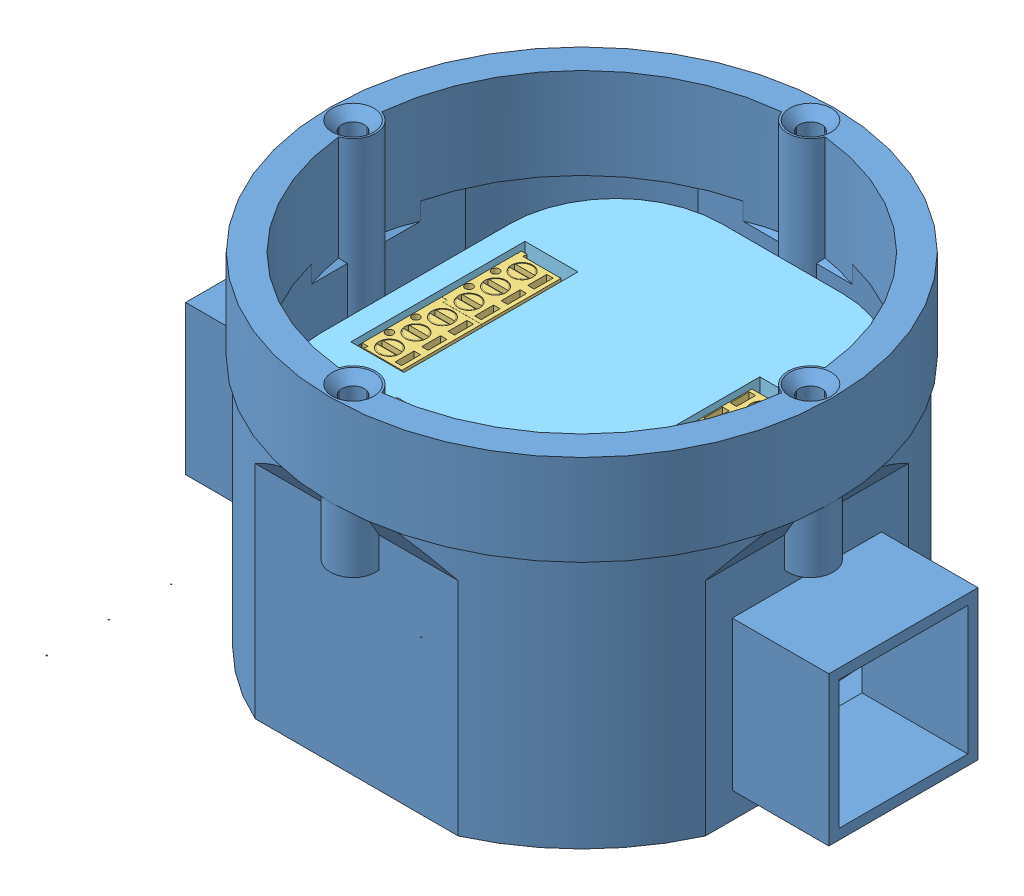
SolidWorks assembly Сборка смартбокса в подрозетнике, configuration Default. Lengths in mm.
Overall size (84.94 45.2 92.53).
6 component instances, 5 part files, 4 mates.
Components (placement in the parent):
- Подрозетник, реинкарнация-1: Подрозетник, реинкарнация [Default] at (-100.2738 -11.9044 46.462) size (84.94 45.2 66.4)
- Сборка плат смарт-бокса-1: Сборка плат смарт-бокса [Default] at (-98.3986 -21.5594 77.5072) x (0 0 1) z (0 1 0) size (85.93 44 32.41)
  - Плата смарт-бокса 1-1: Плата смарт-бокса 1 [Default] at (-165.9192 -27.3465 18.5165) size (50.47 38.8 18.8)
  - Плата смарт-бокса 2-1: Плата смарт-бокса 2 [Default] at (-116.116 -27.2195 30.3365) x (1 0 0) z (0 0 1) size (83.29 38.85 21.16)
  - Корпус для смарт-бокса, новая версия-2: Корпус для смарт-бокса, новая версия [Default] at (-31.0453 -1.8751 23.405) x (1 0 0) z (0 -1 0) size (53 27.5 44)
  - Смарт-бокс, крышка-1: Смарт-бокс, крышка [Default] at (-31.0453 -1.8751 37.155) x (1 0 0) z (0 -1 0) size (53 5 44) (hidden)
Mates (geometry in assembly coordinates):
- Coincident1: coincident anti-aligned: plane of Подрозетник, реинкарнация-1 through (-100.2738 -11.9044 46.462) normal (0 1 0); plane of Сборка плат смарт-бокса-1/Корпус для смарт-бокса, новая версия-2 through (-92.2738 -11.9044 33.962) normal (0 -1 0)
- Parallel1: parallel anti-aligned: plane of Подрозетник, реинкарнация-1 through (-71.7738 20.0956 33.3241) normal (-1 0 0); plane of Сборка плат смарт-бокса-1/Корпус для смарт-бокса, новая версия-2 through (-78.2738 15.5956 58.962) normal (1 0 0)
- Width1: width anti-aligned: plane of Подрозетник, реинкарнация-1 through (-113.4116 20.0956 17.962) normal (0 0 1); plane of Подрозетник, реинкарнация-1 through (-113.4116 20.0956 74.962) normal (0 0 -1); plane of Сборка плат смарт-бокса-1/Корпус для смарт-бокса, новая версия-2 through (-92.2738 15.5956 19.962) normal (0 0 -1); plane of Сборка плат смарт-бокса-1/Корпус для смарт-бокса, новая версия-2 through (-108.2738 15.5956 72.962) normal (0 0 1)
- Width2: width anti-aligned: plane of Подрозетник, реинкарнация-1 through (-71.7738 20.0956 33.3241) normal (-1 0 0); plane of Подрозетник, реинкарнация-1 through (-128.7738 20.0956 33.3241) normal (1 0 0); plane of Сборка плат смарт-бокса-1/Корпус для смарт-бокса, новая версия-2 through (-78.2738 15.5956 58.962) normal (1 0 0); plane of Сборка плат смарт-бокса-1/Корпус для смарт-бокса, новая версия-2 through (-122.2738 15.5956 33.962) normal (-1 0 0)
